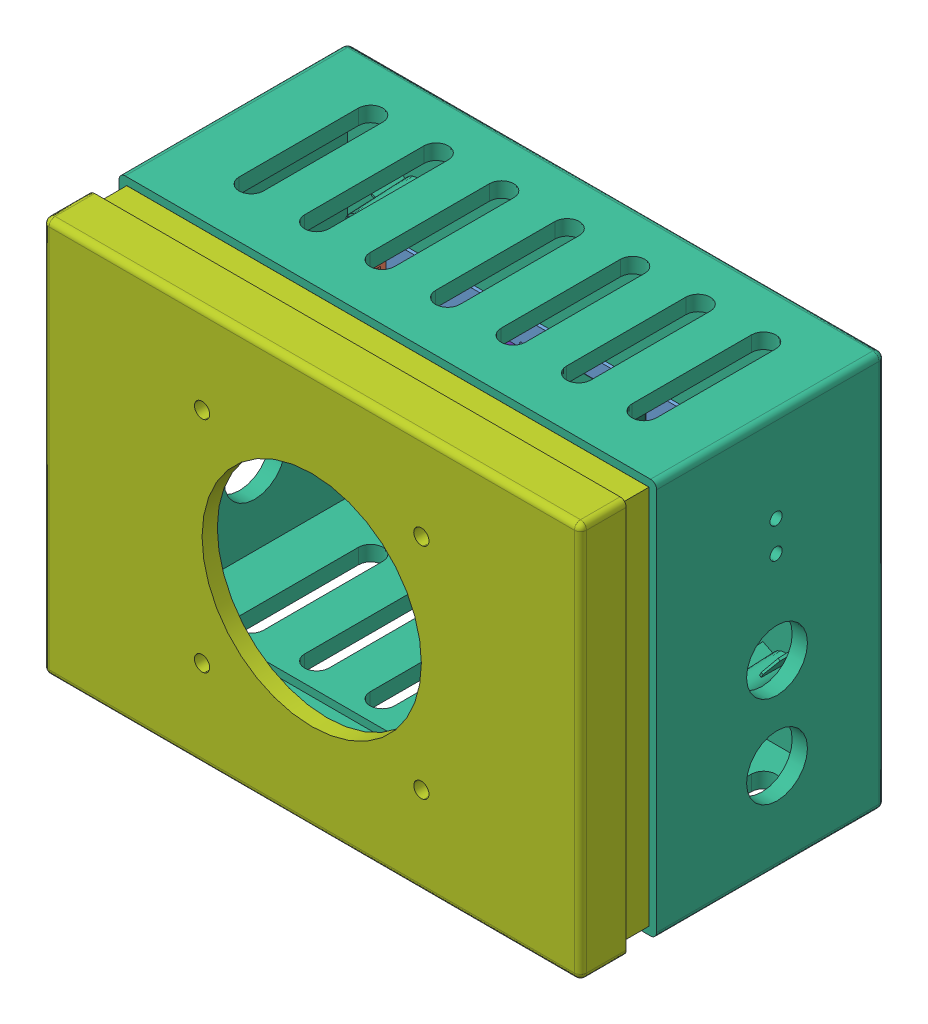
SolidWorks assembly LeadAcidBatteryChargerEnclosure, configuration Default. Lengths in mm.
Overall size (176.49 129.88 100).
840 component instances, 61 part files, 8 mates.
Components (placement in the parent):
- leld acid charger anthima eka.step-1: leld acid charger anthima eka.step [Default] at origin size (126.49 79.88 39.76)
  - Board.step-1: Board.step [Default] at origin size (126.49 79.88 1.1)
    - Open CASCADE STEP translator 7.5 446.1.1.step-1: Open CASCADE STEP translator 7.5 446.1.1.step [Default] at (0 0 -1.1) size (126.49 79.88 1.1)
  - Pwr.step-1: Pwr.step [Default] at origin size (8.1 10.66 13.9)
    - LS_5.08_02_90_3.5SN_OR_BX_1912520000.step-1: LS_5.08_02_90_3.5SN_OR_BX_1912520000.step [Default] at (12.686 74.803 0.0122) x (0 -1 0) z (-1 0 0) size (10.66 13.9 8.1)
  - Battery.step-1: Battery.step [Default] at origin size (8.1 10.66 13.9)
    - LS_5.08_02_90_3.5SN_OR_BX_1912520000.step-1: LS_5.08_02_90_3.5SN_OR_BX_1912520000.step [Default] at (12.178 29.21 0.0122) x (0 -1 0) z (-1 0 0) size (10.66 13.9 8.1)
  - VR3.step-1: VR3.step [Default] at origin size (6.6 6.99 19.06)
    - Res_Bourns_3362P-1-102TLF_eec.step-1: Res_Bourns_3362P-1-102TLF_eec.step [Default] at (37.719 9.744 0) x (1 0 0) z (0 0 1) size (6.6 6.99 19.06)
      - terminal.step-1: terminal.step [Default] at origin size (5.54 3 5)
      - body.step-1: body.step [Default] at origin size (6.6 6.99 5.13)
      - logo.step-1: logo.step [Default] at (0 0 5.13) size (6.02 5.76 0)
      - knob.step-1: knob.step [Default] at origin size (4.98 4.98 9.93)
  - VR2.step-1: VR2.step [Default] at origin size (6.6 6.99 19.06)
    - Res_Bourns_3362P-1-102TLF_eec.step-1: Res_Bourns_3362P-1-102TLF_eec.step [Default] at (28.448 9.906 0) x (1 0 0) z (0 0 1) size (6.6 6.99 19.06)
      - terminal.step-1: terminal.step [Default] at origin size (5.54 3 5)
      - body.step-1: body.step [Default] at origin size (6.6 6.99 5.13)
      - logo.step-1: logo.step [Default] at (0 0 5.13) size (6.02 5.76 0)
      - knob.step-1: knob.step [Default] at origin size (4.98 4.98 9.93)
  - VR1.step-1: VR1.step [Default] at origin size (6.6 6.99 19.06)
    - Res_Bourns_3362P-1-102TLF_eec.step-1: Res_Bourns_3362P-1-102TLF_eec.step [Default] at (46.99 9.525 0) size (6.6 6.99 19.06)
      - terminal.step-1: terminal.step [Default] at origin size (5.54 3 5)
      - body.step-1: body.step [Default] at origin size (6.6 6.99 5.13)
      - logo.step-1: logo.step [Default] at (0 0 5.13) size (6.02 5.76 0)
      - knob.step-1: knob.step [Default] at origin size (4.98 4.98 9.93)
  - U4.step-1: U4.step [Default] at origin size (19.95 7.92 6.68)
    - 8269410800.step-1: 8269410800.step [Default] at (77.851 41.529 0) size (1.1 0.3 2.58)
      - Extruded.step-1: Extruded.step [Default] at origin size (1.1 0.3 2.58)
    - 7386986352.step-1: 7386986352.step [Default] at (77.851 41.499 2.58) size (1.1 0.36 0.3)
      - Extruded-0.step-1: Extruded-0.step [Default] at origin size (1.1 0.36 0.3)
    - 6402678080.step-1: 6402678080.step [Default] at (77.851 41.529 -1.6) size (0.8 0.3 1.6)
      - Extruded-1.step-1: Extruded-1.step [Default] at origin size (0.8 0.3 1.6)
    - 8269410800.step-2: 8269410800.step [Default] at (75.311 41.529 0) size (1.1 0.3 2.58)
      - Extruded.step-1: Extruded.step [Default] at origin size (1.1 0.3 2.58)
    - 7386986352.step-2: 7386986352.step [Default] at (75.311 41.499 2.58) size (1.1 0.36 0.3)
      - Extruded-0.step-1: Extruded-0.step [Default] at origin size (1.1 0.36 0.3)
    - 6402678080.step-2: 6402678080.step [Default] at (75.311 41.529 -1.6) size (0.8 0.3 1.6)
      - Extruded-1.step-1: Extruded-1.step [Default] at origin size (0.8 0.3 1.6)
    - 8269410800.step-3: 8269410800.step [Default] at (72.771 41.529 0) size (1.1 0.3 2.58)
      - Extruded.step-1: Extruded.step [Default] at origin size (1.1 0.3 2.58)
    - 7386986352.step-3: 7386986352.step [Default] at (72.771 41.499 2.58) size (1.1 0.36 0.3)
      - Extruded-0.step-1: Extruded-0.step [Default] at origin size (1.1 0.36 0.3)
    - 6402678080.step-3: 6402678080.step [Default] at (72.771 41.529 -1.6) size (0.8 0.3 1.6)
      - Extruded-1.step-1: Extruded-1.step [Default] at origin size (0.8 0.3 1.6)
    - 8269410800.step-4: 8269410800.step [Default] at (70.231 41.529 0) size (1.1 0.3 2.58)
      - Extruded.step-1: Extruded.step [Default] at origin size (1.1 0.3 2.58)
    - 7386986352.step-4: 7386986352.step [Default] at (70.231 41.499 2.58) size (1.1 0.36 0.3)
      - Extruded-0.step-1: Extruded-0.step [Default] at origin size (1.1 0.36 0.3)
    - 6402678080.step-4: 6402678080.step [Default] at (70.231 41.529 -1.6) size (0.8 0.3 1.6)
      - Extruded-1.step-1: Extruded-1.step [Default] at origin size (0.8 0.3 1.6)
    - 8269410800.step-5: 8269410800.step [Default] at (67.691 41.529 0) size (1.1 0.3 2.58)
      - Extruded.step-1: Extruded.step [Default] at origin size (1.1 0.3 2.58)
    - 7386986352.step-5: 7386986352.step [Default] at (67.691 41.499 2.58) size (1.1 0.36 0.3)
      - Extruded-0.step-1: Extruded-0.step [Default] at origin size (1.1 0.36 0.3)
    - 6402678080.step-5: 6402678080.step [Default] at (67.691 41.529 -1.6) size (0.8 0.3 1.6)
      - Extruded-1.step-1: Extruded-1.step [Default] at origin size (0.8 0.3 1.6)
    - 8269410800.step-6: 8269410800.step [Default] at (65.151 41.529 0) size (1.1 0.3 2.58)
      - Extruded.step-1: Extruded.step [Default] at origin size (1.1 0.3 2.58)
    - 7386986352.step-6: 7386986352.step [Default] at (65.151 41.499 2.58) size (1.1 0.36 0.3)
      - Extruded-0.step-1: Extruded-0.step [Default] at origin size (1.1 0.36 0.3)
    - 6402678080.step-6: 6402678080.step [Default] at (65.151 41.529 -1.6) size (0.8 0.3 1.6)
      - Extruded-1.step-1: Extruded-1.step [Default] at origin size (0.8 0.3 1.6)
    - 8269410800.step-7: 8269410800.step [Default] at (62.611 41.529 0) size (1.1 0.3 2.58)
      - Extruded.step-1: Extruded.step [Default] at origin size (1.1 0.3 2.58)
    - 7386986352.step-7: 7386986352.step [Default] at (62.611 41.499 2.58) size (1.1 0.36 0.3)
      - Extruded-0.step-1: Extruded-0.step [Default] at origin size (1.1 0.36 0.3)
    - 6402678080.step-7: 6402678080.step [Default] at (62.611 41.529 -1.6) size (0.8 0.3 1.6)
      - Extruded-1.step-1: Extruded-1.step [Default] at origin size (0.8 0.3 1.6)
    - 8269410800.step-8: 8269410800.step [Default] at (62.611 33.909 0) size (1.1 0.3 2.58)
      - Extruded.step-1: Extruded.step [Default] at origin size (1.1 0.3 2.58)
    - 7386986352.step-8: 7386986352.step [Default] at (62.611 33.939 2.58) size (1.1 0.36 0.3)
      - Extruded-0.step-1: Extruded-0.step [Default] at origin size (1.1 0.36 0.3)
    - 6402678080.step-8: 6402678080.step [Default] at (62.611 33.909 -1.6) size (0.8 0.3 1.6)
      - Extruded-1.step-1: Extruded-1.step [Default] at origin size (0.8 0.3 1.6)
    - 8269410800.step-9: 8269410800.step [Default] at (65.151 33.909 0) size (1.1 0.3 2.58)
      - Extruded.step-1: Extruded.step [Default] at origin size (1.1 0.3 2.58)
    - 7386986352.step-9: 7386986352.step [Default] at (65.151 33.939 2.58) size (1.1 0.36 0.3)
      - Extruded-0.step-1: Extruded-0.step [Default] at origin size (1.1 0.36 0.3)
    - 6402678080.step-9: 6402678080.step [Default] at (65.151 33.909 -1.6) size (0.8 0.3 1.6)
      - Extruded-1.step-1: Extruded-1.step [Default] at origin size (0.8 0.3 1.6)
    - 8269410800.step-10: 8269410800.step [Default] at (67.691 33.909 0) size (1.1 0.3 2.58)
      - Extruded.step-1: Extruded.step [Default] at origin size (1.1 0.3 2.58)
    - 7386986352.step-10: 7386986352.step [Default] at (67.691 33.939 2.58) size (1.1 0.36 0.3)
      - Extruded-0.step-1: Extruded-0.step [Default] at origin size (1.1 0.36 0.3)
    - 6402678080.step-10: 6402678080.step [Default] at (67.691 33.909 -1.6) size (0.8 0.3 1.6)
      - Extruded-1.step-1: Extruded-1.step [Default] at origin size (0.8 0.3 1.6)
    - 8269410800.step-11: 8269410800.step [Default] at (70.231 33.909 0) size (1.1 0.3 2.58)
      - Extruded.step-1: Extruded.step [Default] at origin size (1.1 0.3 2.58)
    - 7386986352.step-11: 7386986352.step [Default] at (70.231 33.939 2.58) size (1.1 0.36 0.3)
      - Extruded-0.step-1: Extruded-0.step [Default] at origin size (1.1 0.36 0.3)
    - 6402678080.step-11: 6402678080.step [Default] at (70.231 33.909 -1.6) size (0.8 0.3 1.6)
      - Extruded-1.step-1: Extruded-1.step [Default] at origin size (0.8 0.3 1.6)
    - 8269410800.step-12: 8269410800.step [Default] at (72.771 33.909 0) size (1.1 0.3 2.58)
      - Extruded.step-1: Extruded.step [Default] at origin size (1.1 0.3 2.58)
    - 7386986352.step-12: 7386986352.step [Default] at (72.771 33.939 2.58) size (1.1 0.36 0.3)
      - Extruded-0.step-1: Extruded-0.step [Default] at origin size (1.1 0.36 0.3)
    - 6402678080.step-12: 6402678080.step [Default] at (72.771 33.909 -1.6) size (0.8 0.3 1.6)
      - Extruded-1.step-1: Extruded-1.step [Default] at origin size (0.8 0.3 1.6)
    - 8269410800.step-13: 8269410800.step [Default] at (75.311 33.909 0) size (1.1 0.3 2.58)
      - Extruded.step-1: Extruded.step [Default] at origin size (1.1 0.3 2.58)
    - 7386986352.step-13: 7386986352.step [Default] at (75.311 33.939 2.58) size (1.1 0.36 0.3)
      - Extruded-0.step-1: Extruded-0.step [Default] at origin size (1.1 0.36 0.3)
    - 6402678080.step-13: 6402678080.step [Default] at (75.311 33.909 -1.6) size (0.8 0.3 1.6)
      - Extruded-1.step-1: Extruded-1.step [Default] at origin size (0.8 0.3 1.6)
    - 8269410800.step-14: 8269410800.step [Default] at (77.851 33.909 0) size (1.1 0.3 2.58)
      - Extruded.step-1: Extruded.step [Default] at origin size (1.1 0.3 2.58)
    - 7386986352.step-14: 7386986352.step [Default] at (77.851 33.939 2.58) size (1.1 0.36 0.3)
      - Extruded-0.step-1: Extruded-0.step [Default] at origin size (1.1 0.36 0.3)
    - 6402678080.step-14: 6402678080.step [Default] at (77.851 33.909 -1.6) size (0.8 0.3 1.6)
      - Extruded-1.step-1: Extruded-1.step [Default] at origin size (0.8 0.3 1.6)
    - 9083006928.step-1: 9083006928.step [Default] at (70.231 37.719 0.38) size (19.95 7.2 4.7)
      - Extruded-2.step-1: Extruded-2.step [Default] at origin size (19.95 7.2 4.7)
  - U3.step-1: U3.step [Default] at origin size (19.95 7.92 6.68)
    - 8269410800.step-1: 8269410800.step [Default] at (102.743 26.035 0) size (1.1 0.3 2.58)
      - Extruded.step-1: Extruded.step [Default] at origin size (1.1 0.3 2.58)
    - 7386986352.step-1: 7386986352.step [Default] at (102.743 26.005 2.58) size (1.1 0.36 0.3)
      - Extruded-0.step-1: Extruded-0.step [Default] at origin size (1.1 0.36 0.3)
    - 6402678080.step-1: 6402678080.step [Default] at (102.743 26.035 -1.6) size (0.8 0.3 1.6)
      - Extruded-1.step-1: Extruded-1.step [Default] at origin size (0.8 0.3 1.6)
    - 8269410800.step-2: 8269410800.step [Default] at (100.203 26.035 0) size (1.1 0.3 2.58)
      - Extruded.step-1: Extruded.step [Default] at origin size (1.1 0.3 2.58)
    - 7386986352.step-2: 7386986352.step [Default] at (100.203 26.005 2.58) size (1.1 0.36 0.3)
      - Extruded-0.step-1: Extruded-0.step [Default] at origin size (1.1 0.36 0.3)
    - 6402678080.step-2: 6402678080.step [Default] at (100.203 26.035 -1.6) size (0.8 0.3 1.6)
      - Extruded-1.step-1: Extruded-1.step [Default] at origin size (0.8 0.3 1.6)
    - 8269410800.step-3: 8269410800.step [Default] at (97.663 26.035 0) size (1.1 0.3 2.58)
      - Extruded.step-1: Extruded.step [Default] at origin size (1.1 0.3 2.58)
    - 7386986352.step-3: 7386986352.step [Default] at (97.663 26.005 2.58) size (1.1 0.36 0.3)
      - Extruded-0.step-1: Extruded-0.step [Default] at origin size (1.1 0.36 0.3)
    - 6402678080.step-3: 6402678080.step [Default] at (97.663 26.035 -1.6) size (0.8 0.3 1.6)
      - Extruded-1.step-1: Extruded-1.step [Default] at origin size (0.8 0.3 1.6)
    - 8269410800.step-4: 8269410800.step [Default] at (95.123 26.035 0) size (1.1 0.3 2.58)
      - Extruded.step-1: Extruded.step [Default] at origin size (1.1 0.3 2.58)
    - 7386986352.step-4: 7386986352.step [Default] at (95.123 26.005 2.58) size (1.1 0.36 0.3)
      - Extruded-0.step-1: Extruded-0.step [Default] at origin size (1.1 0.36 0.3)
    - 6402678080.step-4: 6402678080.step [Default] at (95.123 26.035 -1.6) size (0.8 0.3 1.6)
      - Extruded-1.step-1: Extruded-1.step [Default] at origin size (0.8 0.3 1.6)
    - 8269410800.step-5: 8269410800.step [Default] at (92.583 26.035 0) size (1.1 0.3 2.58)
      - Extruded.step-1: Extruded.step [Default] at origin size (1.1 0.3 2.58)
    - 7386986352.step-5: 7386986352.step [Default] at (92.583 26.005 2.58) size (1.1 0.36 0.3)
      - Extruded-0.step-1: Extruded-0.step [Default] at origin size (1.1 0.36 0.3)
    - 6402678080.step-5: 6402678080.step [Default] at (92.583 26.035 -1.6) size (0.8 0.3 1.6)
      - Extruded-1.step-1: Extruded-1.step [Default] at origin size (0.8 0.3 1.6)
    - 8269410800.step-6: 8269410800.step [Default] at (90.043 26.035 0) size (1.1 0.3 2.58)
      - Extruded.step-1: Extruded.step [Default] at origin size (1.1 0.3 2.58)
    - 7386986352.step-6: 7386986352.step [Default] at (90.043 26.005 2.58) size (1.1 0.36 0.3)
      - Extruded-0.step-1: Extruded-0.step [Default] at origin size (1.1 0.36 0.3)
    - 6402678080.step-6: 6402678080.step [Default] at (90.043 26.035 -1.6) size (0.8 0.3 1.6)
      - Extruded-1.step-1: Extruded-1.step [Default] at origin size (0.8 0.3 1.6)
    - 8269410800.step-7: 8269410800.step [Default] at (87.503 26.035 0) size (1.1 0.3 2.58)
      - Extruded.step-1: Extruded.step [Default] at origin size (1.1 0.3 2.58)
    - 7386986352.step-7: 7386986352.step [Default] at (87.503 26.005 2.58) size (1.1 0.36 0.3)
      - Extruded-0.step-1: Extruded-0.step [Default] at origin size (1.1 0.36 0.3)
    - 6402678080.step-7: 6402678080.step [Default] at (87.503 26.035 -1.6) size (0.8 0.3 1.6)
      - Extruded-1.step-1: Extruded-1.step [Default] at origin size (0.8 0.3 1.6)
    - 8269410800.step-8: 8269410800.step [Default] at (87.503 18.415 0) size (1.1 0.3 2.58)
      - Extruded.step-1: Extruded.step [Default] at origin size (1.1 0.3 2.58)
    - 7386986352.step-8: 7386986352.step [Default] at (87.503 18.445 2.58) size (1.1 0.36 0.3)
      - Extruded-0.step-1: Extruded-0.step [Default] at origin size (1.1 0.36 0.3)
    - 6402678080.step-8: 6402678080.step [Default] at (87.503 18.415 -1.6) size (0.8 0.3 1.6)
      - Extruded-1.step-1: Extruded-1.step [Default] at origin size (0.8 0.3 1.6)
    - 8269410800.step-9: 8269410800.step [Default] at (90.043 18.415 0) size (1.1 0.3 2.58)
      - Extruded.step-1: Extruded.step [Default] at origin size (1.1 0.3 2.58)
    - 7386986352.step-9: 7386986352.step [Default] at (90.043 18.445 2.58) size (1.1 0.36 0.3)
      - Extruded-0.step-1: Extruded-0.step [Default] at origin size (1.1 0.36 0.3)
    - 6402678080.step-9: 6402678080.step [Default] at (90.043 18.415 -1.6) size (0.8 0.3 1.6)
      - Extruded-1.step-1: Extruded-1.step [Default] at origin size (0.8 0.3 1.6)
    - 8269410800.step-10: 8269410800.step [Default] at (92.583 18.415 0) size (1.1 0.3 2.58)
      - Extruded.step-1: Extruded.step [Default] at origin size (1.1 0.3 2.58)
    - 7386986352.step-10: 7386986352.step [Default] at (92.583 18.445 2.58) size (1.1 0.36 0.3)
      - Extruded-0.step-1: Extruded-0.step [Default] at origin size (1.1 0.36 0.3)
    - 6402678080.step-10: 6402678080.step [Default] at (92.583 18.415 -1.6) size (0.8 0.3 1.6)
      - Extruded-1.step-1: Extruded-1.step [Default] at origin size (0.8 0.3 1.6)
    - 8269410800.step-11: 8269410800.step [Default] at (95.123 18.415 0) size (1.1 0.3 2.58)
      - Extruded.step-1: Extruded.step [Default] at origin size (1.1 0.3 2.58)
    - 7386986352.step-11: 7386986352.step [Default] at (95.123 18.445 2.58) size (1.1 0.36 0.3)
      - Extruded-0.step-1: Extruded-0.step [Default] at origin size (1.1 0.36 0.3)
    - 6402678080.step-11: 6402678080.step [Default] at (95.123 18.415 -1.6) size (0.8 0.3 1.6)
      - Extruded-1.step-1: Extruded-1.step [Default] at origin size (0.8 0.3 1.6)
    - 8269410800.step-12: 8269410800.step [Default] at (97.663 18.415 0) size (1.1 0.3 2.58)
      - Extruded.step-1: Extruded.step [Default] at origin size (1.1 0.3 2.58)
    - 7386986352.step-12: 7386986352.step [Default] at (97.663 18.445 2.58) size (1.1 0.36 0.3)
      - Extruded-0.step-1: Extruded-0.step [Default] at origin size (1.1 0.36 0.3)
    - 6402678080.step-12: 6402678080.step [Default] at (97.663 18.415 -1.6) size (0.8 0.3 1.6)
      - Extruded-1.step-1: Extruded-1.step [Default] at origin size (0.8 0.3 1.6)
    - 8269410800.step-13: 8269410800.step [Default] at (100.203 18.415 0) size (1.1 0.3 2.58)
      - Extruded.step-1: Extruded.step [Default] at origin size (1.1 0.3 2.58)
    - 7386986352.step-13: 7386986352.step [Default] at (100.203 18.445 2.58) size (1.1 0.36 0.3)
      - Extruded-0.step-1: Extruded-0.step [Default] at origin size (1.1 0.36 0.3)
    - 6402678080.step-13: 6402678080.step [Default] at (100.203 18.415 -1.6) size (0.8 0.3 1.6)
      - Extruded-1.step-1: Extruded-1.step [Default] at origin size (0.8 0.3 1.6)
    - 8269410800.step-14: 8269410800.step [Default] at (102.743 18.415 0) size (1.1 0.3 2.58)
      - Extruded.step-1: Extruded.step [Default] at origin size (1.1 0.3 2.58)
    - 7386986352.step-14: 7386986352.step [Default] at (102.743 18.445 2.58) size (1.1 0.36 0.3)
      - Extruded-0.step-1: Extruded-0.step [Default] at origin size (1.1 0.36 0.3)
    - 6402678080.step-14: 6402678080.step [Default] at (102.743 18.415 -1.6) size (0.8 0.3 1.6)
      - Extruded-1.step-1: Extruded-1.step [Default] at origin size (0.8 0.3 1.6)
    - 9083006928.step-1: 9083006928.step [Default] at (95.123 22.225 0.38) size (19.95 7.2 4.7)
      - Extruded-2.step-1: Extruded-2.step [Default] at origin size (19.95 7.2 4.7)
  - U2.step-1: U2.step [Default] at origin size (19.95 7.92 6.68)
    - 8269410800.step-1: 8269410800.step [Default] at (54.102 26.289 0) size (1.1 0.3 2.58)
      - Extruded.step-1: Extruded.step [Default] at origin size (1.1 0.3 2.58)
    - 7386986352.step-1: 7386986352.step [Default] at (54.102 26.259 2.58) size (1.1 0.36 0.3)
      - Extruded-0.step-1: Extruded-0.step [Default] at origin size (1.1 0.36 0.3)
    - 6402678080.step-1: 6402678080.step [Default] at (54.102 26.289 -1.6) size (0.8 0.3 1.6)
      - Extruded-1.step-1: Extruded-1.step [Default] at origin size (0.8 0.3 1.6)
    - 8269410800.step-2: 8269410800.step [Default] at (51.562 26.289 0) size (1.1 0.3 2.58)
      - Extruded.step-1: Extruded.step [Default] at origin size (1.1 0.3 2.58)
    - 7386986352.step-2: 7386986352.step [Default] at (51.562 26.259 2.58) size (1.1 0.36 0.3)
      - Extruded-0.step-1: Extruded-0.step [Default] at origin size (1.1 0.36 0.3)
    - 6402678080.step-2: 6402678080.step [Default] at (51.562 26.289 -1.6) size (0.8 0.3 1.6)
      - Extruded-1.step-1: Extruded-1.step [Default] at origin size (0.8 0.3 1.6)
    - 8269410800.step-3: 8269410800.step [Default] at (49.022 26.289 0) size (1.1 0.3 2.58)
      - Extruded.step-1: Extruded.step [Default] at origin size (1.1 0.3 2.58)
    - 7386986352.step-3: 7386986352.step [Default] at (49.022 26.259 2.58) size (1.1 0.36 0.3)
      - Extruded-0.step-1: Extruded-0.step [Default] at origin size (1.1 0.36 0.3)
    - 6402678080.step-3: 6402678080.step [Default] at (49.022 26.289 -1.6) size (0.8 0.3 1.6)
      - Extruded-1.step-1: Extruded-1.step [Default] at origin size (0.8 0.3 1.6)
    - 8269410800.step-4: 8269410800.step [Default] at (46.482 26.289 0) size (1.1 0.3 2.58)
      - Extruded.step-1: Extruded.step [Default] at origin size (1.1 0.3 2.58)
    - 7386986352.step-4: 7386986352.step [Default] at (46.482 26.259 2.58) size (1.1 0.36 0.3)
      - Extruded-0.step-1: Extruded-0.step [Default] at origin size (1.1 0.36 0.3)
    - 6402678080.step-4: 6402678080.step [Default] at (46.482 26.289 -1.6) size (0.8 0.3 1.6)
      - Extruded-1.step-1: Extruded-1.step [Default] at origin size (0.8 0.3 1.6)
    - 8269410800.step-5: 8269410800.step [Default] at (43.942 26.289 0) size (1.1 0.3 2.58)
      - Extruded.step-1: Extruded.step [Default] at origin size (1.1 0.3 2.58)
    - 7386986352.step-5: 7386986352.step [Default] at (43.942 26.259 2.58) size (1.1 0.36 0.3)
      - Extruded-0.step-1: Extruded-0.step [Default] at origin size (1.1 0.36 0.3)
    - 6402678080.step-5: 6402678080.step [Default] at (43.942 26.289 -1.6) size (0.8 0.3 1.6)
      - Extruded-1.step-1: Extruded-1.step [Default] at origin size (0.8 0.3 1.6)
    - 8269410800.step-6: 8269410800.step [Default] at (41.402 26.289 0) size (1.1 0.3 2.58)
      - Extruded.step-1: Extruded.step [Default] at origin size (1.1 0.3 2.58)
    - 7386986352.step-6: 7386986352.step [Default] at (41.402 26.259 2.58) size (1.1 0.36 0.3)
      - Extruded-0.step-1: Extruded-0.step [Default] at origin size (1.1 0.36 0.3)
    - 6402678080.step-6: 6402678080.step [Default] at (41.402 26.289 -1.6) size (0.8 0.3 1.6)
      - Extruded-1.step-1: Extruded-1.step [Default] at origin size (0.8 0.3 1.6)
    - 8269410800.step-7: 8269410800.step [Default] at (38.862 26.289 0) size (1.1 0.3 2.58)
      - Extruded.step-1: Extruded.step [Default] at origin size (1.1 0.3 2.58)
    - 7386986352.step-7: 7386986352.step [Default] at (38.862 26.259 2.58) size (1.1 0.36 0.3)
      - Extruded-0.step-1: Extruded-0.step [Default] at origin size (1.1 0.36 0.3)
    - 6402678080.step-7: 6402678080.step [Default] at (38.862 26.289 -1.6) size (0.8 0.3 1.6)
      - Extruded-1.step-1: Extruded-1.step [Default] at origin size (0.8 0.3 1.6)
    - 8269410800.step-8: 8269410800.step [Default] at (38.862 18.669 0) size (1.1 0.3 2.58)
      - Extruded.step-1: Extruded.step [Default] at origin size (1.1 0.3 2.58)
    - 7386986352.step-8: 7386986352.step [Default] at (38.862 18.699 2.58) size (1.1 0.36 0.3)
      - Extruded-0.step-1: Extruded-0.step [Default] at origin size (1.1 0.36 0.3)
    - 6402678080.step-8: 6402678080.step [Default] at (38.862 18.669 -1.6) size (0.8 0.3 1.6)
      - Extruded-1.step-1: Extruded-1.step [Default] at origin size (0.8 0.3 1.6)
    - 8269410800.step-9: 8269410800.step [Default] at (41.402 18.669 0) size (1.1 0.3 2.58)
      - Extruded.step-1: Extruded.step [Default] at origin size (1.1 0.3 2.58)
    - 7386986352.step-9: 7386986352.step [Default] at (41.402 18.699 2.58) size (1.1 0.36 0.3)
      - Extruded-0.step-1: Extruded-0.step [Default] at origin size (1.1 0.36 0.3)
    - 6402678080.step-9: 6402678080.step [Default] at (41.402 18.669 -1.6) size (0.8 0.3 1.6)
      - Extruded-1.step-1: Extruded-1.step [Default] at origin size (0.8 0.3 1.6)
    - 8269410800.step-10: 8269410800.step [Default] at (43.942 18.669 0) size (1.1 0.3 2.58)
      - Extruded.step-1: Extruded.step [Default] at origin size (1.1 0.3 2.58)
    - 7386986352.step-10: 7386986352.step [Default] at (43.942 18.699 2.58) size (1.1 0.36 0.3)
      - Extruded-0.step-1: Extruded-0.step [Default] at origin size (1.1 0.36 0.3)
    - 6402678080.step-10: 6402678080.step [Default] at (43.942 18.669 -1.6) size (0.8 0.3 1.6)
      - Extruded-1.step-1: Extruded-1.step [Default] at origin size (0.8 0.3 1.6)
    - 8269410800.step-11: 8269410800.step [Default] at (46.482 18.669 0) size (1.1 0.3 2.58)
      - Extruded.step-1: Extruded.step [Default] at origin size (1.1 0.3 2.58)
    - 7386986352.step-11: 7386986352.step [Default] at (46.482 18.699 2.58) size (1.1 0.36 0.3)
      - Extruded-0.step-1: Extruded-0.step [Default] at origin size (1.1 0.36 0.3)
    - 6402678080.step-11: 6402678080.step [Default] at (46.482 18.669 -1.6) size (0.8 0.3 1.6)
      - Extruded-1.step-1: Extruded-1.step [Default] at origin size (0.8 0.3 1.6)
    - 8269410800.step-12: 8269410800.step [Default] at (49.022 18.669 0) size (1.1 0.3 2.58)
      - Extruded.step-1: Extruded.step [Default] at origin size (1.1 0.3 2.58)
    - 7386986352.step-12: 7386986352.step [Default] at (49.022 18.699 2.58) size (1.1 0.36 0.3)
      - Extruded-0.step-1: Extruded-0.step [Default] at origin size (1.1 0.36 0.3)
    - 6402678080.step-12: 6402678080.step [Default] at (49.022 18.669 -1.6) size (0.8 0.3 1.6)
      - Extruded-1.step-1: Extruded-1.step [Default] at origin size (0.8 0.3 1.6)
    - 8269410800.step-13: 8269410800.step [Default] at (51.562 18.669 0) size (1.1 0.3 2.58)
      - Extruded.step-1: Extruded.step [Default] at origin size (1.1 0.3 2.58)
    - 7386986352.step-13: 7386986352.step [Default] at (51.562 18.699 2.58) size (1.1 0.36 0.3)
      - Extruded-0.step-1: Extruded-0.step [Default] at origin size (1.1 0.36 0.3)
    - 6402678080.step-13: 6402678080.step [Default] at (51.562 18.669 -1.6) size (0.8 0.3 1.6)
      - Extruded-1.step-1: Extruded-1.step [Default] at origin size (0.8 0.3 1.6)
    - 8269410800.step-14: 8269410800.step [Default] at (54.102 18.669 0) size (1.1 0.3 2.58)
      - Extruded.step-1: Extruded.step [Default] at origin size (1.1 0.3 2.58)
    - 7386986352.step-14: 7386986352.step [Default] at (54.102 18.699 2.58) size (1.1 0.36 0.3)
      - Extruded-0.step-1: Extruded-0.step [Default] at origin size (1.1 0.36 0.3)
    - 6402678080.step-14: 6402678080.step [Default] at (54.102 18.669 -1.6) size (0.8 0.3 1.6)
      - Extruded-1.step-1: Extruded-1.step [Default] at origin size (0.8 0.3 1.6)
    - 9083006928.step-1: 9083006928.step [Default] at (46.482 22.479 0.38) size (19.95 7.2 4.7)
      - Extruded-2.step-1: Extruded-2.step [Default] at origin size (19.95 7.2 4.7)
  - U1.step-1: U1.step [Default] at origin size (19.95 7.92 6.68)
    - 8269410800.step-1: 8269410800.step [Default] at (77.978 26.035 0) size (1.1 0.3 2.58)
      - Extruded.step-1: Extruded.step [Default] at origin size (1.1 0.3 2.58)
    - 7386986352.step-1: 7386986352.step [Default] at (77.978 26.005 2.58) size (1.1 0.36 0.3)
      - Extruded-0.step-1: Extruded-0.step [Default] at origin size (1.1 0.36 0.3)
    - 6402678080.step-1: 6402678080.step [Default] at (77.978 26.035 -1.6) size (0.8 0.3 1.6)
      - Extruded-1.step-1: Extruded-1.step [Default] at origin size (0.8 0.3 1.6)
    - 8269410800.step-2: 8269410800.step [Default] at (75.438 26.035 0) size (1.1 0.3 2.58)
      - Extruded.step-1: Extruded.step [Default] at origin size (1.1 0.3 2.58)
    - 7386986352.step-2: 7386986352.step [Default] at (75.438 26.005 2.58) size (1.1 0.36 0.3)
      - Extruded-0.step-1: Extruded-0.step [Default] at origin size (1.1 0.36 0.3)
    - 6402678080.step-2: 6402678080.step [Default] at (75.438 26.035 -1.6) size (0.8 0.3 1.6)
      - Extruded-1.step-1: Extruded-1.step [Default] at origin size (0.8 0.3 1.6)
    - 8269410800.step-3: 8269410800.step [Default] at (72.898 26.035 0) size (1.1 0.3 2.58)
      - Extruded.step-1: Extruded.step [Default] at origin size (1.1 0.3 2.58)
    - 7386986352.step-3: 7386986352.step [Default] at (72.898 26.005 2.58) size (1.1 0.36 0.3)
      - Extruded-0.step-1: Extruded-0.step [Default] at origin size (1.1 0.36 0.3)
    - 6402678080.step-3: 6402678080.step [Default] at (72.898 26.035 -1.6) size (0.8 0.3 1.6)
      - Extruded-1.step-1: Extruded-1.step [Default] at origin size (0.8 0.3 1.6)
    - 8269410800.step-4: 8269410800.step [Default] at (70.358 26.035 0) size (1.1 0.3 2.58)
      - Extruded.step-1: Extruded.step [Default] at origin size (1.1 0.3 2.58)
    - 7386986352.step-4: 7386986352.step [Default] at (70.358 26.005 2.58) size (1.1 0.36 0.3)
      - Extruded-0.step-1: Extruded-0.step [Default] at origin size (1.1 0.36 0.3)
    - 6402678080.step-4: 6402678080.step [Default] at (70.358 26.035 -1.6) size (0.8 0.3 1.6)
      - Extruded-1.step-1: Extruded-1.step [Default] at origin size (0.8 0.3 1.6)
    - 8269410800.step-5: 8269410800.step [Default] at (67.818 26.035 0) size (1.1 0.3 2.58)
      - Extruded.step-1: Extruded.step [Default] at origin size (1.1 0.3 2.58)
    - 7386986352.step-5: 7386986352.step [Default] at (67.818 26.005 2.58) size (1.1 0.36 0.3)
      - Extruded-0.step-1: Extruded-0.step [Default] at origin size (1.1 0.36 0.3)
    - 6402678080.step-5: 6402678080.step [Default] at (67.818 26.035 -1.6) size (0.8 0.3 1.6)
      - Extruded-1.step-1: Extruded-1.step [Default] at origin size (0.8 0.3 1.6)
    - 8269410800.step-6: 8269410800.step [Default] at (65.278 26.035 0) size (1.1 0.3 2.58)
      - Extruded.step-1: Extruded.step [Default] at origin size (1.1 0.3 2.58)
    - 7386986352.step-6: 7386986352.step [Default] at (65.278 26.005 2.58) size (1.1 0.36 0.3)
      - Extruded-0.step-1: Extruded-0.step [Default] at origin size (1.1 0.36 0.3)
    - 6402678080.step-6: 6402678080.step [Default] at (65.278 26.035 -1.6) size (0.8 0.3 1.6)
      - Extruded-1.step-1: Extruded-1.step [Default] at origin size (0.8 0.3 1.6)
    - 8269410800.step-7: 8269410800.step [Default] at (62.738 26.035 0) size (1.1 0.3 2.58)
      - Extruded.step-1: Extruded.step [Default] at origin size (1.1 0.3 2.58)
    - 7386986352.step-7: 7386986352.step [Default] at (62.738 26.005 2.58) size (1.1 0.36 0.3)
      - Extruded-0.step-1: Extruded-0.step [Default] at origin size (1.1 0.36 0.3)
    - 6402678080.step-7: 6402678080.step [Default] at (62.738 26.035 -1.6) size (0.8 0.3 1.6)
      - Extruded-1.step-1: Extruded-1.step [Default] at origin size (0.8 0.3 1.6)
    - 8269410800.step-8: 8269410800.step [Default] at (62.738 18.415 0) size (1.1 0.3 2.58)
      - Extruded.step-1: Extruded.step [Default] at origin size (1.1 0.3 2.58)
    - 7386986352.step-8: 7386986352.step [Default] at (62.738 18.445 2.58) size (1.1 0.36 0.3)
      - Extruded-0.step-1: Extruded-0.step [Default] at origin size (1.1 0.36 0.3)
    - 6402678080.step-8: 6402678080.step [Default] at (62.738 18.415 -1.6) size (0.8 0.3 1.6)
      - Extruded-1.step-1: Extruded-1.step [Default] at origin size (0.8 0.3 1.6)
    - 8269410800.step-9: 8269410800.step [Default] at (65.278 18.415 0) size (1.1 0.3 2.58)
      - Extruded.step-1: Extruded.step [Default] at origin size (1.1 0.3 2.58)
    - 7386986352.step-9: 7386986352.step [Default] at (65.278 18.445 2.58) size (1.1 0.36 0.3)
      - Extruded-0.step-1: Extruded-0.step [Default] at origin size (1.1 0.36 0.3)
    - 6402678080.step-9: 6402678080.step [Default] at (65.278 18.415 -1.6) size (0.8 0.3 1.6)
      - Extruded-1.step-1: Extruded-1.step [Default] at origin size (0.8 0.3 1.6)
    - 8269410800.step-10: 8269410800.step [Default] at (67.818 18.415 0) size (1.1 0.3 2.58)
      - Extruded.step-1: Extruded.step [Default] at origin size (1.1 0.3 2.58)
    - 7386986352.step-10: 7386986352.step [Default] at (67.818 18.445 2.58) size (1.1 0.36 0.3)
      - Extruded-0.step-1: Extruded-0.step [Default] at origin size (1.1 0.36 0.3)
    - 6402678080.step-10: 6402678080.step [Default] at (67.818 18.415 -1.6) size (0.8 0.3 1.6)
      - Extruded-1.step-1: Extruded-1.step [Default] at origin size (0.8 0.3 1.6)
    - 8269410800.step-11: 8269410800.step [Default] at (70.358 18.415 0) size (1.1 0.3 2.58)
      - Extruded.step-1: Extruded.step [Default] at origin size (1.1 0.3 2.58)
    - 7386986352.step-11: 7386986352.step [Default] at (70.358 18.445 2.58) size (1.1 0.36 0.3)
      - Extruded-0.step-1: Extruded-0.step [Default] at origin size (1.1 0.36 0.3)
    - 6402678080.step-11: 6402678080.step [Default] at (70.358 18.415 -1.6) size (0.8 0.3 1.6)
      - Extruded-1.step-1: Extruded-1.step [Default] at origin size (0.8 0.3 1.6)
    - 8269410800.step-12: 8269410800.step [Default] at (72.898 18.415 0) size (1.1 0.3 2.58)
      - Extruded.step-1: Extruded.step [Default] at origin size (1.1 0.3 2.58)
    - 7386986352.step-12: 7386986352.step [Default] at (72.898 18.445 2.58) size (1.1 0.36 0.3)
      - Extruded-0.step-1: Extruded-0.step [Default] at origin size (1.1 0.36 0.3)
    - 6402678080.step-12: 6402678080.step [Default] at (72.898 18.415 -1.6) size (0.8 0.3 1.6)
      - Extruded-1.step-1: Extruded-1.step [Default] at origin size (0.8 0.3 1.6)
    - 8269410800.step-13: 8269410800.step [Default] at (75.438 18.415 0) size (1.1 0.3 2.58)
      - Extruded.step-1: Extruded.step [Default] at origin size (1.1 0.3 2.58)
    - 7386986352.step-13: 7386986352.step [Default] at (75.438 18.445 2.58) size (1.1 0.36 0.3)
      - Extruded-0.step-1: Extruded-0.step [Default] at origin size (1.1 0.36 0.3)
    - 6402678080.step-13: 6402678080.step [Default] at (75.438 18.415 -1.6) size (0.8 0.3 1.6)
      - Extruded-1.step-1: Extruded-1.step [Default] at origin size (0.8 0.3 1.6)
    - 8269410800.step-14: 8269410800.step [Default] at (77.978 18.415 0) size (1.1 0.3 2.58)
      - Extruded.step-1: Extruded.step [Default] at origin size (1.1 0.3 2.58)
    - 7386986352.step-14: 7386986352.step [Default] at (77.978 18.445 2.58) size (1.1 0.36 0.3)
      - Extruded-0.step-1: Extruded-0.step [Default] at origin size (1.1 0.36 0.3)
    - 6402678080.step-14: 6402678080.step [Default] at (77.978 18.415 -1.6) size (0.8 0.3 1.6)
      - Extruded-1.step-1: Extruded-1.step [Default] at origin size (0.8 0.3 1.6)
    - 9083006928.step-1: 9083006928.step [Default] at (70.358 22.225 0.38) size (19.95 7.2 4.7)
      - Extruded-2.step-1: Extruded-2.step [Default] at origin size (19.95 7.2 4.7)
  - R25.step-1: R25.step [Default] at origin size (2.5 10.6 6.5)
    - Res_Vishay_MRS25-1K5_eec.step-1: Res_Vishay_MRS25-1K5_eec.step [Default] at (50.927 38.481 0) x (0 1 0) z (0 0 1) size (10.6 2.5 6.5)
      - 1.step-1: 1.step [Default] at origin size (6.5 2.5 2.5)
      - 2.step-1: 2.step [Default] at origin size (10.6 0.6 5.55)
      - Vishay.step-1: Vishay.step [Default] at (-3.2314 -0.0636 1.2909) x (0 -1 0) z (-1 0 0) size (0.59 0.5 0.02)
  - R24.step-1: R24.step [Default] at origin size (10.6 2.5 6.5)
    - Res_Vishay_MRS25-1K5_eec.step-1: Res_Vishay_MRS25-1K5_eec.step [Default] at (75.946 12.573 0) x (-1 0 0) z (0 0 1) size (10.6 2.5 6.5)
      - 1.step-1: 1.step [Default] at origin size (6.5 2.5 2.5)
      - 2.step-1: 2.step [Default] at origin size (10.6 0.6 5.55)
      - Vishay.step-1: Vishay.step [Default] at (-3.2314 -0.0636 1.2909) x (0 -1 0) z (-1 0 0) size (0.59 0.5 0.02)
  - R23.step-1: R23.step [Default] at origin size (2.5 10.6 6.5)
    - Res_Vishay_MRS25-1K5_eec.step-1: Res_Vishay_MRS25-1K5_eec.step [Default] at (22.098 24.13 0) x (0 -1 0) z (0 0 1) size (10.6 2.5 6.5)
      - 1.step-1: 1.step [Default] at origin size (6.5 2.5 2.5)
      - 2.step-1: 2.step [Default] at origin size (10.6 0.6 5.55)
      - Vishay.step-1: Vishay.step [Default] at (-3.2314 -0.0636 1.2909) x (0 -1 0) z (-1 0 0) size (0.59 0.5 0.02)
  - R22.step-1: R22.step [Default] at origin size (10.6 2.5 6.5)
    - Res_Vishay_MRS25-1K5_eec.step-1: Res_Vishay_MRS25-1K5_eec.step [Default] at (90.805 12.7 0) x (-1 0 0) z (0 0 1) size (10.6 2.5 6.5)
      - 1.step-1: 1.step [Default] at origin size (6.5 2.5 2.5)
      - 2.step-1: 2.step [Default] at origin size (10.6 0.6 5.55)
      - Vishay.step-1: Vishay.step [Default] at (-3.2314 -0.0636 1.2909) x (0 -1 0) z (-1 0 0) size (0.59 0.5 0.02)
  - R21.step-1: R21.step [Default] at origin size (2.5 10.6 6.5)
    - Res_Vishay_MRS25-1K5_eec.step-1: Res_Vishay_MRS25-1K5_eec.step [Default] at (27.305 24.003 0) x (0 1 0) z (0 0 1) size (10.6 2.5 6.5)
      - 1.step-1: 1.step [Default] at origin size (6.5 2.5 2.5)
      - 2.step-1: 2.step [Default] at origin size (10.6 0.6 5.55)
      - Vishay.step-1: Vishay.step [Default] at (-3.2314 -0.0636 1.2909) x (0 -1 0) z (-1 0 0) size (0.59 0.5 0.02)
  - R20.step-1: R20.step [Default] at origin size (10.6 2.5 6.5)
    - Res_Vishay_MRS25-1K5_eec.step-1: Res_Vishay_MRS25-1K5_eec.step [Default] at (90.551 6.477 0) x (1 0 0) z (0 0 1) size (10.6 2.5 6.5)
      - 1.step-1: 1.step [Default] at origin size (6.5 2.5 2.5)
      - 2.step-1: 2.step [Default] at origin size (10.6 0.6 5.55)
      - Vishay.step-1: Vishay.step [Default] at (-3.2314 -0.0636 1.2909) x (0 -1 0) z (-1 0 0) size (0.59 0.5 0.02)
  - R19.step-1: R19.step [Default] at origin size (29.91 9.5 14)
    - Res_Yageo_SQP500JB-1R2_eec.step-1: Res_Yageo_SQP500JB-1R2_eec.step [Default] at (87.249 69.596 0) x (1 0 0) z (0 0 1) size (29.91 9.5 14)
      - 1-3.step-1: 1-3.step [Default] at origin size (29.91 0.8 9.4)
      - 2-4.step-1: 2-4.step [Default] at origin size (22 9.5 10)
      - Yageo Logo.step-1: Yageo Logo.step [Default] at (-8.1443 3.6121 9.991) size (4.52 1.05 0.01)
  - R18.step-1: R18.step [Default] at origin size (29.91 9.5 14)
    - Res_Yageo_SQP500JB-1R2_eec.step-1: Res_Yageo_SQP500JB-1R2_eec.step [Default] at (87.553 54.229 0) x (1 0 0) z (0 0 1) size (29.91 9.5 14)
      - 1-3.step-1: 1-3.step [Default] at origin size (29.91 0.8 9.4)
      - 2-4.step-1: 2-4.step [Default] at origin size (22 9.5 10)
      - Yageo Logo.step-1: Yageo Logo.step [Default] at (-8.1443 3.6121 9.991) size (4.52 1.05 0.01)
  - R16.step-1: R16.step [Default] at origin size (2.5 10.6 6.5)
    - Res_Vishay_MRS25-1K5_eec.step-1: Res_Vishay_MRS25-1K5_eec.step [Default] at (42.799 54.991 0) x (0 1 0) z (0 0 1) size (10.6 2.5 6.5)
      - 1.step-1: 1.step [Default] at origin size (6.5 2.5 2.5)
      - 2.step-1: 2.step [Default] at origin size (10.6 0.6 5.55)
      - Vishay.step-1: Vishay.step [Default] at (-3.2314 -0.0636 1.2909) x (0 -1 0) z (-1 0 0) size (0.59 0.5 0.02)
  - R15.step-1: R15.step [Default] at origin size (9.5 29.91 14)
    - Res_Yageo_SQP500JB-1R2_eec.step-1: Res_Yageo_SQP500JB-1R2_eec.step [Default] at (114.173 22.479 0) x (0 1 0) z (0 0 1) size (29.91 9.5 14)
      - 1-3.step-1: 1-3.step [Default] at origin size (29.91 0.8 9.4)
      - 2-4.step-1: 2-4.step [Default] at origin size (22 9.5 10)
      - Yageo Logo.step-1: Yageo Logo.step [Default] at (-8.1443 3.6121 9.991) size (4.52 1.05 0.01)
  - R14.step-1: R14.step [Default] at origin size (10.6 2.5 6.5)
    - Res_Vishay_MRS25-1K5_eec.step-1: Res_Vishay_MRS25-1K5_eec.step [Default] at (76.327 6.858 0) x (-1 0 0) z (0 0 1) size (10.6 2.5 6.5)
      - 1.step-1: 1.step [Default] at origin size (6.5 2.5 2.5)
      - 2.step-1: 2.step [Default] at origin size (10.6 0.6 5.55)
      - Vishay.step-1: Vishay.step [Default] at (-3.2314 -0.0636 1.2909) x (0 -1 0) z (-1 0 0) size (0.59 0.5 0.02)
  - R13.step-1: R13.step [Default] at origin size (2.5 10.6 6.5)
    - Res_Vishay_MRS25-1K5_eec.step-1: Res_Vishay_MRS25-1K5_eec.step [Default] at (31.877 24.003 0) x (0 1 0) z (0 0 1) size (10.6 2.5 6.5)
      - 1.step-1: 1.step [Default] at origin size (6.5 2.5 2.5)
      - 2.step-1: 2.step [Default] at origin size (10.6 0.6 5.55)
      - Vishay.step-1: Vishay.step [Default] at (-3.2314 -0.0636 1.2909) x (0 -1 0) z (-1 0 0) size (0.59 0.5 0.02)
  - R11.step-1: R11.step [Default] at origin size (10.6 2.5 6.5)
    - Res_Vishay_MRS25-1K5_eec.step-1: Res_Vishay_MRS25-1K5_eec.step [Default] at (14.859 13.208 0) x (1 0 0) z (0 0 1) size (10.6 2.5 6.5)
      - 1.step-1: 1.step [Default] at origin size (6.5 2.5 2.5)
      - 2.step-1: 2.step [Default] at origin size (10.6 0.6 5.55)
      - Vishay.step-1: Vishay.step [Default] at (-3.2314 -0.0636 1.2909) x (0 -1 0) z (-1 0 0) size (0.59 0.5 0.02)
  - R10.step-1: R10.step [Default] at origin size (10.6 2.5 6.5)
    - Res_Vishay_MRS25-1K5_eec.step-1: Res_Vishay_MRS25-1K5_eec.step [Default] at (14.732 7.874 0) x (1 0 0) z (0 0 1) size (10.6 2.5 6.5)
      - 1.step-1: 1.step [Default] at origin size (6.5 2.5 2.5)
      - 2.step-1: 2.step [Default] at origin size (10.6 0.6 5.55)
      - Vishay.step-1: Vishay.step [Default] at (-3.2314 -0.0636 1.2909) x (0 -1 0) z (-1 0 0) size (0.59 0.5 0.02)
  - R9.step-1: R9.step [Default] at origin size (2.5 10.6 6.5)
    - Res_Vishay_MRS25-1K5_eec.step-1: Res_Vishay_MRS25-1K5_eec.step [Default] at (107.696 48.895 0) x (0 1 0) z (0 0 1) size (10.6 2.5 6.5)
      - 1.step-1: 1.step [Default] at origin size (6.5 2.5 2.5)
      - 2.step-1: 2.step [Default] at origin size (10.6 0.6 5.55)
      - Vishay.step-1: Vishay.step [Default] at (-3.2314 -0.0636 1.2909) x (0 -1 0) z (-1 0 0) size (0.59 0.5 0.02)
  - R8.step-1: R8.step [Default] at origin size (2.5 10.6 6.5)
    - Res_Vishay_MRS25-1K5_eec.step-1: Res_Vishay_MRS25-1K5_eec.step [Default] at (113.665 49.276 0) x (0 1 0) z (0 0 1) size (10.6 2.5 6.5)
      - 1.step-1: 1.step [Default] at origin size (6.5 2.5 2.5)
      - 2.step-1: 2.step [Default] at origin size (10.6 0.6 5.55)
      - Vishay.step-1: Vishay.step [Default] at (-3.2314 -0.0636 1.2909) x (0 -1 0) z (-1 0 0) size (0.59 0.5 0.02)
  - R5.step-1: R5.step [Default] at origin size (2.5 10.6 6.5)
    - Res_Vishay_MRS25-1K5_eec.step-1: Res_Vishay_MRS25-1K5_eec.step [Default] at (33.02 40.005 0) x (0 -1 0) z (0 0 1) size (10.6 2.5 6.5)
      - 1.step-1: 1.step [Default] at origin size (6.5 2.5 2.5)
      - 2.step-1: 2.step [Default] at origin size (10.6 0.6 5.55)
      - Vishay.step-1: Vishay.step [Default] at (-3.2314 -0.0636 1.2909) x (0 -1 0) z (-1 0 0) size (0.59 0.5 0.02)
  - R4.step-1: R4.step [Default] at origin size (2.5 10.6 6.5)
    - Res_Vishay_MRS25-1K5_eec.step-1: Res_Vishay_MRS25-1K5_eec.step [Default] at (28.194 40.005 0) x (0 -1 0) z (0 0 1) size (10.6 2.5 6.5)
      - 1.step-1: 1.step [Default] at origin size (6.5 2.5 2.5)
      - 2.step-1: 2.step [Default] at origin size (10.6 0.6 5.55)
      - Vishay.step-1: Vishay.step [Default] at (-3.2314 -0.0636 1.2909) x (0 -1 0) z (-1 0 0) size (0.59 0.5 0.02)
  - R3.step-1: R3.step [Default] at origin size (2.5 10.6 6.5)
    - Res_Vishay_MRS25-1K5_eec.step-1: Res_Vishay_MRS25-1K5_eec.step [Default] at (14.732 39.878 0) x (0 1 0) z (0 0 1) size (10.6 2.5 6.5)
      - 1.step-1: 1.step [Default] at origin size (6.5 2.5 2.5)
      - 2.step-1: 2.step [Default] at origin size (10.6 0.6 5.55)
      - Vishay.step-1: Vishay.step [Default] at (-3.2314 -0.0636 1.2909) x (0 -1 0) z (-1 0 0) size (0.59 0.5 0.02)
  - R2.step-1: R2.step [Default] at origin size (2.5 10.6 6.5)
    - Res_Vishay_MRS25-1K5_eec.step-1: Res_Vishay_MRS25-1K5_eec.step [Default] at (11.303 55.118 0) x (0 -1 0) z (0 0 1) size (10.6 2.5 6.5)
      - 1.step-1: 1.step [Default] at origin size (6.5 2.5 2.5)
      - 2.step-1: 2.step [Default] at origin size (10.6 0.6 5.55)
      - Vishay.step-1: Vishay.step [Default] at (-3.2314 -0.0636 1.2909) x (0 -1 0) z (-1 0 0) size (0.59 0.5 0.02)
  - R1.step-1: R1.step [Default] at origin size (2.5 10.6 6.5)
    - Res_Vishay_MRS25-1K5_eec.step-1: Res_Vishay_MRS25-1K5_eec.step [Default] at (6.477 54.991 0) x (0 1 0) z (0 0 1) size (10.6 2.5 6.5)
      - 1.step-1: 1.step [Default] at origin size (6.5 2.5 2.5)
      - 2.step-1: 2.step [Default] at origin size (10.6 0.6 5.55)
      - Vishay.step-1: Vishay.step [Default] at (-3.2314 -0.0636 1.2909) x (0 -1 0) z (-1 0 0) size (0.59 0.5 0.02)
  - Q2.step-1: Q2.step [Default] at origin size (4.85 10.3 21.45)
    - 6853938128.step-1: 6853938128.step [Default] at (45.085 36.957 0) size (0.5 1.34 2.8)
      - Extruded-5.step-1: Extruded-5.step [Default] at origin size (0.5 1.34 2.8)
    - 6853937968.step-1: 6853937968.step [Default] at (45.085 36.957 -1.6) size (0.5 0.78 1.6)
      - Extruded-6.step-1: Extruded-6.step [Default] at origin size (0.5 0.78 1.6)
    - 6853938128.step-2: 6853938128.step [Default] at (45.085 39.497 0) size (0.5 1.34 2.8)
      - Extruded-5.step-1: Extruded-5.step [Default] at origin size (0.5 1.34 2.8)
    - 6853937968.step-2: 6853937968.step [Default] at (45.085 39.497 -1.6) size (0.5 0.78 1.6)
      - Extruded-6.step-1: Extruded-6.step [Default] at origin size (0.5 0.78 1.6)
    - 6853938128.step-3: 6853938128.step [Default] at (45.085 42.037 0) size (0.5 1.34 2.8)
      - Extruded-5.step-1: Extruded-5.step [Default] at origin size (0.5 1.34 2.8)
    - 6853937968.step-3: 6853937968.step [Default] at (45.085 42.037 -1.6) size (0.5 0.78 1.6)
      - Extruded-6.step-1: Extruded-6.step [Default] at origin size (0.5 0.78 1.6)
    - 6853937488.step-1: 6853937488.step [Default] at (44.84 39.497 2.8) size (4.85 10.3 10.85)
      - Extruded-7.step-1: Extruded-7.step [Default] at origin size (4.85 10.3 10.85)
    - 6853937248.step-1: 6853937248.step [Default] at (43.04 39.497 13.65) size (1.25 9.95 1.48)
      - Extruded-8.step-1: Extruded-8.step [Default] at origin size (1.25 9.95 1.48)
    - 6853937088.step-1: 6853937088.step [Default] at (43.04 36.8217 15.13) size (1.25 4.6 0.04)
      - Extruded-9.step-1: Extruded-9.step [Default] at origin size (1.25 4.6 0.04)
    - 6853937088.step-2: 6853937088.step [Default] at (43.04 42.1723 15.13) size (1.25 4.6 0.04)
      - Extruded-9.step-1: Extruded-9.step [Default] at origin size (1.25 4.6 0.04)
    - 6853937088.step-3: 6853937088.step [Default] at (43.04 36.8217 18.94) size (1.25 4.6 0.04)
